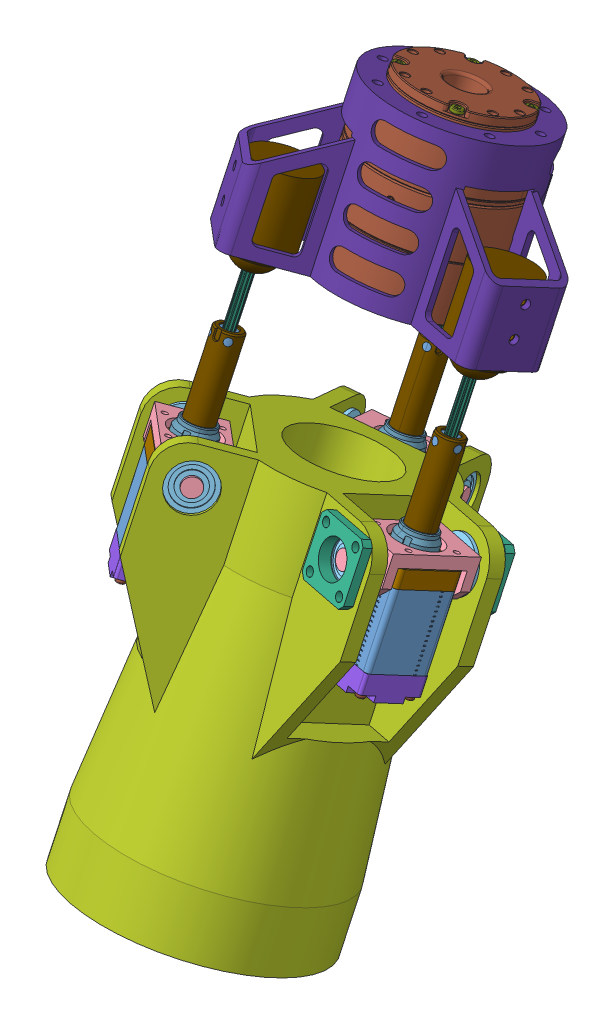
SolidWorks assembly 机械臂总装, configuration 默认. Lengths in mm.
Overall size (121.27 258.43 202.88).
175 component instances, 61 part files, 56 mates.
Components (placement in the parent):
- CRA-RI40-52-PRO-XX 2023.5.4 - Drum-1: CRA-RI40-52-PRO-XX 2023.5.4 - Drum [默认] at (-65.3352 0.778 -52.4868) x (-0.773511 0.267701 0.574471) z (-0.632199 -0.261859 -0.729215) size (67.95 60.31 67.96)
  - CRA-RI40-52-PRO-XX 2023.5.4 - Drum.stp-1: CRA-RI40-52-PRO-XX 2023.5.4 - Drum.stp [默认] at origin size (67.95 60.31 67.96)
    - CRA-RI40-52-PRO-XX_1_ASM.stp-1: CRA-RI40-52-PRO-XX_1_ASM.stp [默认] at origin size (67.95 60.31 67.96)
      - XB11-52__10001_ASM.stp-1: XB11-52__10001_ASM.stp [默认] at (0 16.8 0) x (0.703875 0 -0.710324) z (-0.710324 0 -0.703875) size (66.32 0.8 66.32)
        - XB11-52-06__10001.stp-1: XB11-52-06__10001.stp [默认] at (0 15.8 0) x (0.791272 0 -0.611464) z (-0.611464 0 -0.791272) size (47.28 0.81 47.28)
      - TINYMBS20WITHCONNECTOR2_ASM.stp-1: TINYMBS20WITHCONNECTOR2_ASM.stp [默认] at (2.7275 -27.9719 -6.5848) x (0 -1 0) z (0.92388 0 0.382683) size (0.82 3.25 5.53)
        - FH34SRJ8S05SH_STEP_STEP_ASM.stp-1: FH34SRJ8S05SH_STEP_STEP_ASM.stp [默认] at (-6.4719 -22.2833 0) x (0 0 -1) z (1 0 0) size (5.53 3.25 0.82)
          - NONE-51348.stp-1: NONE-51348.stp [默认] at origin size (0.15 0.3 0.08)
          - NONE-53783.stp-1: NONE-53783.stp [默认] at origin size (0.15 0.3 0.08)
          - NONE-55744.stp-1: NONE-55744.stp [默认] at origin size (0.15 0.08 0.08)
          - NONE-57763.stp-1: NONE-57763.stp [默认] at origin size (0.15 0.08 0.08)
          - NONE-60582.stp-1: NONE-60582.stp [默认] at origin size (0.15 0.3 0.08)
          - NONE-60979.stp-1: NONE-60979.stp [默认] at origin size (0.15 0.3 0.08)
          - NONE-62950.stp-1: NONE-62950.stp [默认] at origin size (0.15 0.3 0.08)
          - NONE-64179.stp-1: NONE-64179.stp [默认] at origin size (0.15 0.3 0.08)
          - NONE-65774.stp-1: NONE-65774.stp [默认] at origin size (0.15 0.08 0.08)
          - NONE-66548.stp-1: NONE-66548.stp [默认] at origin size (0.15 0.35 0.23)
          - NONE-67775.stp-1: NONE-67775.stp [默认] at origin size (0.15 0.35 0.23)
          - NONE-133224.stp-1: NONE-133224.stp [默认] at origin size (0.15 0.08 0.08)
          - NONE-134873.stp-1: NONE-134873.stp [默认] at origin size (0.15 0.3 0.08)
          - NONE-136443.stp-1: NONE-136443.stp [默认] at origin size (0.15 0.08 0.08)
          - NONE-141250.stp-1: NONE-141250.stp [默认] at origin size (0.15 0.35 0.23)
          - NONE-145287.stp-1: NONE-145287.stp [默认] at origin size (0.15 0.08 0.08)
          - NONE-147294.stp-1: NONE-147294.stp [默认] at origin size (0.15 0.08 0.08)
          - NONE-214429.stp-1: NONE-214429.stp [默认] at origin size (0.15 0.9 0.82)
          - NONE-214822.stp-1: NONE-214822.stp [默认] at origin size (0.15 0.3 0.08)
          - NONE-215190.stp-1: NONE-215190.stp [默认] at origin size (0.15 0.08 0.08)
          - NONE-216041.stp-1: NONE-216041.stp [默认] at origin size (0.15 0.35 0.23)
          - NONE-217624.stp-1: NONE-217624.stp [默认] at origin size (0.15 0.35 0.23)
          - NONE-222885.stp-1: NONE-222885.stp [默认] at origin size (0.15 0.35 0.23)
          - NONE-224875.stp-1: NONE-224875.stp [默认] at origin size (0.15 0.35 0.23)
          - NONE-228113.stp-1: NONE-228113.stp [默认] at origin size (0.15 0.9 0.82)
          - NONE-228916.stp-1: NONE-228916.stp [默认] at origin size (0.15 0.35 0.23)
      - CROSS_RECESSED_COUNTERSUNK_HE_1.stp-1: CROSS_RECESSED_COUNTERSUNK_HE_1.stp [默认] at (-21.8123 -33.1 2.8703) x (0 1 0) z (0.6 0 0.8) size (4 3.5 3.5)
      - RI40-52-D12-02__1000.stp-1: RI40-52-D12-02__1000.stp [默认] at (0 -15 0) x (0.382683 0 -0.92388) z (0.92388 0 0.382683) size (52.01 56.6 52)
      - CROSS_RECESSED_CHEESE_HEAD_SC_1.stp-1: CROSS_RECESSED_CHEESE_HEAD_SC_1.stp [默认] at (3.9505 15.5 -22.4044) x (0 -1 0) z (1 0 0) size (5.7 2.98 2.98)
      - MC50-D25X12_5_000.stp-1: MC50-D25X12_5_000.stp [默认] at (0.0001 -26.6014 0.0001) x (0.382686 0 -0.923879) z (0 -1 0) size (48.11 50.01 13.43)
      - CROSS_RECESSED_CHEESE_HEAD_SC_1.stp-2: CROSS_RECESSED_CHEESE_HEAD_SC_1.stp [默认] at (-3.9505 15.5 22.4044) x (0 -1 0) z (-1 0 0) size (5.7 2.98 2.98)
      - CROSS_RECESSED_COUNTERSUNK_HE_1.stp-2: CROSS_RECESSED_COUNTERSUNK_HE_1.stp [默认] at (-3.0048 -33.1 22.5417) x (0 1 0) z (0.395734 0 0.918365) size (4 3.5 3.5)
      - CROSS_RECESSED_CHEESE_HEAD_SC_1.stp-3: CROSS_RECESSED_CHEESE_HEAD_SC_1.stp [默认] at (-18.6357 15.5 13.0489) x (0 -1 0) z (-0.707107 0 -0.707107) size (5.7 2.98 2.98)
      - CROSS_RECESSED_COUNTERSUNK_HE_1.stp-3: CROSS_RECESSED_COUNTERSUNK_HE_1.stp [默认] at (18.8645 -33.1 -12.4259) x (0 1 0) z (0.188455 0 0.982082) size (4 3.5 3.5)
      - _M2X3_M2X3_100.stp-1: _M2X3_M2X3_100.stp [默认] at (-21.8118 -29.6014 2.8705) x (0.8 0 -0.6) z (0.6 0 0.8) size (3.23 5.8 2.8)
      - _M2X3_M2X3_100.stp-2: _M2X3_M2X3_100.stp [默认] at (-13.393 -29.6014 -17.4539) x (0.918365 0 -0.395734) z (0.395734 0 0.918365) size (3.23 5.8 2.8)
      - CROSS_RECESSED_CHEESE_HEAD_SC_1.stp-4: CROSS_RECESSED_CHEESE_HEAD_SC_1.stp [默认] at (-22.4044 15.5 -3.9505) x (0 -1 0) z (0 0 -1) size (5.7 2.98 2.98)
      - CROSS_RECESSED_CHEESE_HEAD_SC_1.stp-5: CROSS_RECESSED_CHEESE_HEAD_SC_1.stp [默认] at (13.0489 15.5 18.6357) x (0 -1 0) z (-0.707107 0 0.707107) size (5.7 2.98 2.98)
      - HEXAGON_SOCKET_HEAD_CAP_SCREW_1.stp-1: HEXAGON_SOCKET_HEAD_CAP_SCREW_1.stp [默认] at (19.8197 15.9 12.6265) x (0 -1 0) z (-0.954517 0 0.298155) size (22.5 4.5 4.5)
      - M2-3_10001.stp-1: M2-3_10001.stp [默认] at (0.7742 21 -17.7331) x (0.020141 0 0.999797) z (-0.999797 0 0.020141) size (4 5.4 4)
      - HEXAGON_SOCKET_HEAD_CAP_SCREW_1.stp-2: HEXAGON_SOCKET_HEAD_CAP_SCREW_1.stp [默认] at (-19.8197 15.9 -12.6265) x (0 -1 0) z (0.954517 0 -0.298155) size (22.5 4.5 4.5)
      - CROSS_RECESSED_CHEESE_HEAD_SC_1.stp-6: CROSS_RECESSED_CHEESE_HEAD_SC_1.stp [默认] at (18.6357 15.5 -13.0489) x (0 -1 0) z (0.707107 0 0.707107) size (5.7 2.98 2.98)
      - M2-3_10001.stp-2: M2-3_10001.stp [默认] at (-17.7331 21 -0.7742) x (0.999797 0 -0.020141) z (0.020141 0 0.999797) size (4 5.4 4)
      - _M2X3_M2X3_100.stp-3: _M2X3_M2X3_100.stp [默认] at (-3.0038 -29.6014 22.5414) x (0.982082 0 -0.188455) z (0.188455 0 0.982082) size (3.23 5.8 2.8)
      - M2-3_10001.stp-3: M2-3_10001.stp [默认] at (-0.7742 21 17.7331) x (-0.020141 0 -0.999797) z (0.999797 0 -0.020141) size (4 5.4 4)
      - _M2X3_M2X3_100.stp-4: _M2X3_M2X3_100.stp [默认] at (18.8646 -29.6014 -12.4267) size (3.23 5.8 2.8)
      - CROSS_RECESSED_COUNTERSUNK_HE_1.stp-4: CROSS_RECESSED_COUNTERSUNK_HE_1.stp [默认] at (-13.393 -33.1 -17.4539) x (0 1 0) z (0 0 1) size (4 3.5 3.5)
      - M2-3_10001.stp-4: M2-3_10001.stp [默认] at (17.7331 21 0.7742) x (-0.999797 0 0.020141) z (-0.020141 0 -0.999797) size (4 5.4 4)
      - CROSS_RECESSED_CHEESE_HEAD_SC_1.stp-7: CROSS_RECESSED_CHEESE_HEAD_SC_1.stp [默认] at (22.4044 15.5 3.9505) x (0 -1 0) z (0 0 1) size (5.7 2.98 2.98)
      - CROSS_RECESSED_CHEESE_HEAD_SC_1.stp-8: CROSS_RECESSED_CHEESE_HEAD_SC_1.stp [默认] at (-13.0489 15.5 -18.6357) x (0 -1 0) z (0.707107 0 -0.707107) size (5.7 2.98 2.98)
- 手腕电机座-1: 手腕电机座 [默认] at (-66.8577 -30.748 -39.8459) x (-0.288066 -0.344371 -0.893547) z (0.956563 -0.147114 -0.251684) size (84.79 53 96.67)
- 球铰2-1: 球铰2 [默认] at (-91.8577 2.9201 -23.4423) x (-0.727754 -0.224677 -0.647992) z (-0.684375 0.29959 0.664738) size (21 30.5 20.4)
- 球铰2-2: 球铰2 [默认] at (-28.733 -6.7882 -40.0512) x (-0.228809 0.371791 0.899677) z (0.972441 0.044781 0.228809) size (21 30.5 20.4)
- 球铰2-3: 球铰2 [默认] at (-76.7583 -21.6149 -82.813) x (0.956563 -0.147114 -0.251684) z (-0.288066 -0.344371 -0.893547) size (21 30.5 20.4)
- 20NC38..31-1: 20NC38..31 [默认] at (-34.2487 -117.8316 4.4347) x (0.046372 0.927308 -0.371416) z (0.972366 0.043263 0.229417) size (109.8 25.88 45.74)
  - 20NC38..31.STEP-1: 20NC38..31.STEP [默认] at origin size (109.8 25.88 45.74)
    - 02-20-38.15________.STEP-1: 02-20-38.15________.STEP [默认] at origin size (39.65 25.88 45.74)
      - 02-20-38.STEP-1: 02-20-38.STEP [默认] at (20.075 0 0) x (0 0 1) z (-1 0 0) size (26.04 25.88 31.46)
        - 02-20-24.15_10-20-001-2.STEP-1: 02-20-24.15_10-20-001-2.STEP [默认] at origin size (20 20 24.15)
        - 13-20-8.5____.STEP-1: 13-20-8.5____.STEP [默认] at (0 0 16.075) x (0 1 0) z (0 0 -1) size (18.2 22.2 10.51)
        - 13-20-12.5______.STEP-1: 13-20-12.5______.STEP [默认] at (0 0 -14.575) x (0.707107 0.707107 0) z (0 0 1) size (18.3 18.3 15.8)
      - 03-20-008______38_______default.STEP-1: 03-20-008______38_______default.STEP [默认] at (3.8 0 0) x (1 0 0) z (0 0.78069 0.624918) size (32.3 16.26 16.27)
        - 06-20-008______38_________01-20-007-1.STEP-1: 06-20-008______38_________01-20-007-1.STEP [默认] at origin size (32.3 7 7)
        - 03-20-4.2-6YK_10-20-006-2.STEP-1: 03-20-4.2-6YK_10-20-006-2.STEP [默认] at (24.2 0 0) x (0 0.91534 0.402682) z (-1 0 0) size (12.06 12.08 4.24)
        - 10-20-001__________.STEP-1: 10-20-001__________.STEP [默认] at (16.9 0 0) x (0 0 1) z (-1 0 0) size (11 11 1)
        - 08-20-001______1_______07-20-001-1.STEP-1: 08-20-001______1_______07-20-001-1.STEP [默认] at (22.1 0 0) x (0 0 1) z (-1 0 0) size (11 11 1)
        - 08-20-001______1_______07-20-001-1.STEP-2: 08-20-001______1_______07-20-001-1.STEP [默认] at (11.4 0 0) x (0 0 1) z (-1 0 0) size (11 11 1)
        - 03-20-4.2-6YK_10-20-006-2.STEP-2: 03-20-4.2-6YK_10-20-006-2.STEP [默认] at (19 0 0) x (0 0.888249 0.459362) z (-1 0 0) size (12.06 12.08 4.24)
        - 03-20-4.2-6YK_10-20-006-2.STEP-3: 03-20-4.2-6YK_10-20-006-2.STEP [默认] at (13.5 0 0) x (0 0.91534 0.402682) z (-1 0 0) size (12.06 12.08 4.24)
        - 03-20-4.2-6YK_10-20-006-2.STEP-4: 03-20-4.2-6YK_10-20-006-2.STEP [默认] at (8.3 0 0) x (0 0.888249 0.459362) z (-1 0 0) size (12.06 12.08 4.24)
      - 01-20-003__20__________________.STEP-1: 01-20-003__20__________________.STEP [默认] at origin size (8.8 20 20)
      - 01-20-001__20__________________.STEP-1: 01-20-001__20__________________.STEP [默认] at (31.35 0 0) x (0 0 1) z (1 0 0) size (20 20 8.3)
      - 09-20-001____9X__5X4)_09-20-001.STEP-1: 09-20-001____9X__5X4)_09-20-001.STEP [默认] at (33.1 0 0) x (1 0 0) z (0 0.994502 0.104719) size (3 9 9)
      - 09-20-001____9X__5X4)_09-20-001.STEP-2: 09-20-001____9X__5X4)_09-20-001.STEP [默认] at (3.8 0 0) x (1 0 0) z (0 -0.49427 -0.869308) size (3 9 9)
      - 11-20-002__M2-37__20-42__.STEP-1: 11-20-002__M2-37__20-42__.STEP [默认] at (0.39 -7.7 7.7) x (0 0 -1) z (1 0 0) size (3 3 33)
      - 11-20-002__M2-37__20-42__.STEP-2: 11-20-002__M2-37__20-42__.STEP [默认] at (0.39 -7.7 -7.7) x (0 1 0) z (1 0 0) size (3 3 33)
      - 11-20-002__M2-37__20-42__.STEP-3: 11-20-002__M2-37__20-42__.STEP [默认] at (0.39 7.7 -7.7) x (0 0 1) z (1 0 0) size (3 3 33)
      - 11-20-002__M2-37__20-42__.STEP-4: 11-20-002__M2-37__20-42__.STEP [默认] at (0.39 7.7 7.7) x (0 -1 0) z (1 0 0) size (3 3 33)
      - 06-20-099__20___________20____________YK.STEP-1: 06-20-099__20___________20____________YK.STEP [默认] at (31.1 0 0) x (0 -0.624918 0.78069) z (-1 0 0) size (6.01 6.01 10)
      - 14-20-001__20-28____________________.STEP-1: 14-20-001__20-28____________________.STEP [默认] at (6.15 0 -8.6) x (0 -1 0) z (0 0 1) size (10.5 3.4 24.5)
    - 07-20-007__________________.STEP-1: 07-20-007__________________.STEP [默认] at (39.65 0 0) x (-1 0 0) z (0 -0.999857 -0.016895) size (6 12.92 13)
    - 07-20-013-2______________.STEP-1: 07-20-013-2______________.STEP [默认] at (68.4 0 0) x (0 -0.714016 0.700129) z (1 0 0) size (3.42 3.5 41.4)
    - 07-20-013-3______________.STEP-1: 07-20-013-3______________.STEP [默认] at (20.15 0 0) x (0 0.924225 0.381849) z (1 0 0) size (8 8 56.63)
    - 07-20-006__20______.STEP-1: 07-20-006__20______.STEP [默认] at (67.9 0 0) x (0 0.924225 0.381849) z (1 0 0) size (3.9 4.45 0.4)
    - 07-20-013-1__20_____________08-20-002-1.STEP-1: 07-20-013-1__20_____________08-20-002-1.STEP [默认] at (36.1 0 0) x (0 0.004204 -0.999991) z (1 0 0) size (9.01 9.01 35.91)
    - 07-20-002__20________________.STEP-1: 07-20-002__20________________.STEP [默认] at (69.65 0 0) x (0 0.004204 -0.999991) z (1 0 0) size (9.01 9.01 3.1)
- 螺纹转换套-1: 螺纹转换套 [默认] at (-30.0844 -34.5593 -28.9185) x (-0.195243 -0.356231 -0.913772) z (0.046372 0.927308 -0.371416) size (5 5 5)
- 球-1: 球 [默认] at (-29.7853 -28.5782 -31.3141) x (-0.55453 -0.285367 -0.781705) z (0.830871 -0.242211 -0.500987) size (14 13.45 14)
- 球-2: 球 [默认] at (-92.91 -18.87 -14.7052) x (0.833324 -0.238487 -0.498693) z (0.551058 0.287142 0.783508) size (14 13.45 14)
- 螺纹转换套-2: 螺纹转换套 [默认] at (-78.0965 -49.3819 -71.6684) x (0.952783 0.073148 0.29471) z (0.044309 0.926671 -0.373253) size (5 5 5)
- 螺纹转换套-3: 螺纹转换套 [默认] at (-93.1916 -24.8538 -12.3142) x (-0.196131 -0.355877 -0.91372) z (0.043661 0.927725 -0.370703) size (5 5 5)
- 球-3: 球 [默认] at (-77.8107 -43.4049 -74.0759) x (0.898492 0.126374 0.420407) z (-0.436749 0.353993 0.827006) size (14 13.45 14)
- 20NC38..31-2: 20NC38..31 [默认] at (-82.0754 -132.597 -38.1503) x (0.044309 0.926671 -0.373253) z (-0.288139 -0.345888 -0.892937) size (109.8 25.88 45.74)
  - 20NC38..31.STEP-1: 20NC38..31.STEP [默认] at origin size (109.8 25.88 45.74)
    - 02-20-38.15________.STEP-1: 02-20-38.15________.STEP [默认] at origin size (39.65 25.88 45.74)
      - 02-20-38.STEP-1: 02-20-38.STEP [默认] at (20.075 0 0) x (0 0 1) z (-1 0 0) size (26.04 25.88 31.46)
        - 02-20-24.15_10-20-001-2.STEP-1: 02-20-24.15_10-20-001-2.STEP [默认] at origin size (20 20 24.15)
        - 13-20-8.5____.STEP-1: 13-20-8.5____.STEP [默认] at (0 0 16.075) x (0 1 0) z (0 0 -1) size (18.2 22.2 10.51)
        - 13-20-12.5______.STEP-1: 13-20-12.5______.STEP [默认] at (0 0 -14.575) x (0.707107 0.707107 0) z (0 0 1) size (18.3 18.3 15.8)
      - 03-20-008______38_______default.STEP-1: 03-20-008______38_______default.STEP [默认] at (3.8 0 0) x (1 0 0) z (0 0.78069 0.624918) size (32.3 16.26 16.27)
        - 06-20-008______38_________01-20-007-1.STEP-1: 06-20-008______38_________01-20-007-1.STEP [默认] at origin size (32.3 7 7)
        - 03-20-4.2-6YK_10-20-006-2.STEP-1: 03-20-4.2-6YK_10-20-006-2.STEP [默认] at (24.2 0 0) x (0 0.91534 0.402682) z (-1 0 0) size (12.06 12.08 4.24)
        - 10-20-001__________.STEP-1: 10-20-001__________.STEP [默认] at (16.9 0 0) x (0 0 1) z (-1 0 0) size (11 11 1)
        - 08-20-001______1_______07-20-001-1.STEP-1: 08-20-001______1_______07-20-001-1.STEP [默认] at (22.1 0 0) x (0 0 1) z (-1 0 0) size (11 11 1)
        - 08-20-001______1_______07-20-001-1.STEP-2: 08-20-001______1_______07-20-001-1.STEP [默认] at (11.4 0 0) x (0 0 1) z (-1 0 0) size (11 11 1)
        - 03-20-4.2-6YK_10-20-006-2.STEP-2: 03-20-4.2-6YK_10-20-006-2.STEP [默认] at (19 0 0) x (0 0.888249 0.459362) z (-1 0 0) size (12.06 12.08 4.24)
        - 03-20-4.2-6YK_10-20-006-2.STEP-3: 03-20-4.2-6YK_10-20-006-2.STEP [默认] at (13.5 0 0) x (0 0.91534 0.402682) z (-1 0 0) size (12.06 12.08 4.24)
        - 03-20-4.2-6YK_10-20-006-2.STEP-4: 03-20-4.2-6YK_10-20-006-2.STEP [默认] at (8.3 0 0) x (0 0.888249 0.459362) z (-1 0 0) size (12.06 12.08 4.24)
      - 01-20-003__20__________________.STEP-1: 01-20-003__20__________________.STEP [默认] at origin size (8.8 20 20)
      - 01-20-001__20__________________.STEP-1: 01-20-001__20__________________.STEP [默认] at (31.35 0 0) x (0 0 1) z (1 0 0) size (20 20 8.3)
      - 09-20-001____9X__5X4)_09-20-001.STEP-1: 09-20-001____9X__5X4)_09-20-001.STEP [默认] at (33.1 0 0) x (1 0 0) z (0 0.994502 0.104719) size (3 9 9)
      - 09-20-001____9X__5X4)_09-20-001.STEP-2: 09-20-001____9X__5X4)_09-20-001.STEP [默认] at (3.8 0 0) x (1 0 0) z (0 -0.49427 -0.869308) size (3 9 9)
      - 11-20-002__M2-37__20-42__.STEP-1: 11-20-002__M2-37__20-42__.STEP [默认] at (0.39 -7.7 7.7) x (0 0 -1) z (1 0 0) size (3 3 33)
      - 11-20-002__M2-37__20-42__.STEP-2: 11-20-002__M2-37__20-42__.STEP [默认] at (0.39 -7.7 -7.7) x (0 1 0) z (1 0 0) size (3 3 33)
      - 11-20-002__M2-37__20-42__.STEP-3: 11-20-002__M2-37__20-42__.STEP [默认] at (0.39 7.7 -7.7) x (0 0 1) z (1 0 0) size (3 3 33)
      - 11-20-002__M2-37__20-42__.STEP-4: 11-20-002__M2-37__20-42__.STEP [默认] at (0.39 7.7 7.7) x (0 -1 0) z (1 0 0) size (3 3 33)
      - 06-20-099__20___________20____________YK.STEP-1: 06-20-099__20___________20____________YK.STEP [默认] at (31.1 0 0) x (0 -0.624918 0.78069) z (-1 0 0) size (6.01 6.01 10)
      - 14-20-001__20-28____________________.STEP-1: 14-20-001__20-28____________________.STEP [默认] at (6.15 0 -8.6) x (0 -1 0) z (0 0 1) size (10.5 3.4 24.5)
    - 07-20-007__________________.STEP-1: 07-20-007__________________.STEP [默认] at (39.65 0 0) x (-1 0 0) z (0 -0.999857 -0.016895) size (6 12.92 13)
    - 07-20-013-2______________.STEP-1: 07-20-013-2______________.STEP [默认] at (68.4 0 0) x (0 -0.714016 0.700129) z (1 0 0) size (3.42 3.5 41.4)
    - 07-20-013-3______________.STEP-1: 07-20-013-3______________.STEP [默认] at (20.15 0 0) x (0 0.924225 0.381849) z (1 0 0) size (8 8 56.63)
    - 07-20-006__20______.STEP-1: 07-20-006__20______.STEP [默认] at (67.9 0 0) x (0 0.924225 0.381849) z (1 0 0) size (3.9 4.45 0.4)
    - 07-20-013-1__20_____________08-20-002-1.STEP-1: 07-20-013-1__20_____________08-20-002-1.STEP [默认] at (36.1 0 0) x (0 0.004204 -0.999991) z (1 0 0) size (9.01 9.01 35.91)
    - 07-20-002__20________________.STEP-1: 07-20-002__20________________.STEP [默认] at (69.65 0 0) x (0 0.004204 -0.999991) z (1 0 0) size (9.01 9.01 3.1)
- 20NC38..31-3: 20NC38..31 [默认] at (-97.1124 -108.1635 20.9749) x (0.043661 0.927725 -0.370703) z (-0.684447 0.298072 0.665346) size (109.8 25.88 45.74)
  - 20NC38..31.STEP-1: 20NC38..31.STEP [默认] at origin size (109.8 25.88 45.74)
    - 02-20-38.15________.STEP-1: 02-20-38.15________.STEP [默认] at origin size (39.65 25.88 45.74)
      - 02-20-38.STEP-1: 02-20-38.STEP [默认] at (20.075 0 0) x (0 0 1) z (-1 0 0) size (26.04 25.88 31.46)
        - 02-20-24.15_10-20-001-2.STEP-1: 02-20-24.15_10-20-001-2.STEP [默认] at origin size (20 20 24.15)
        - 13-20-8.5____.STEP-1: 13-20-8.5____.STEP [默认] at (0 0 16.075) x (0 1 0) z (0 0 -1) size (18.2 22.2 10.51)
        - 13-20-12.5______.STEP-1: 13-20-12.5______.STEP [默认] at (0 0 -14.575) x (0.707107 0.707107 0) z (0 0 1) size (18.3 18.3 15.8)
      - 03-20-008______38_______default.STEP-1: 03-20-008______38_______default.STEP [默认] at (3.8 0 0) x (1 0 0) z (0 0.78069 0.624918) size (32.3 16.26 16.27)
        - 06-20-008______38_________01-20-007-1.STEP-1: 06-20-008______38_________01-20-007-1.STEP [默认] at origin size (32.3 7 7)
        - 03-20-4.2-6YK_10-20-006-2.STEP-1: 03-20-4.2-6YK_10-20-006-2.STEP [默认] at (24.2 0 0) x (0 0.91534 0.402682) z (-1 0 0) size (12.06 12.08 4.24)
        - 10-20-001__________.STEP-1: 10-20-001__________.STEP [默认] at (16.9 0 0) x (0 0 1) z (-1 0 0) size (11 11 1)
        - 08-20-001______1_______07-20-001-1.STEP-1: 08-20-001______1_______07-20-001-1.STEP [默认] at (22.1 0 0) x (0 0 1) z (-1 0 0) size (11 11 1)
        - 08-20-001______1_______07-20-001-1.STEP-2: 08-20-001______1_______07-20-001-1.STEP [默认] at (11.4 0 0) x (0 0 1) z (-1 0 0) size (11 11 1)
        - 03-20-4.2-6YK_10-20-006-2.STEP-2: 03-20-4.2-6YK_10-20-006-2.STEP [默认] at (19 0 0) x (0 0.888249 0.459362) z (-1 0 0) size (12.06 12.08 4.24)
        - 03-20-4.2-6YK_10-20-006-2.STEP-3: 03-20-4.2-6YK_10-20-006-2.STEP [默认] at (13.5 0 0) x (0 0.91534 0.402682) z (-1 0 0) size (12.06 12.08 4.24)
        - 03-20-4.2-6YK_10-20-006-2.STEP-4: 03-20-4.2-6YK_10-20-006-2.STEP [默认] at (8.3 0 0) x (0 0.888249 0.459362) z (-1 0 0) size (12.06 12.08 4.24)
      - 01-20-003__20__________________.STEP-1: 01-20-003__20__________________.STEP [默认] at origin size (8.8 20 20)
      - 01-20-001__20__________________.STEP-1: 01-20-001__20__________________.STEP [默认] at (31.35 0 0) x (0 0 1) z (1 0 0) size (20 20 8.3)
      - 09-20-001____9X__5X4)_09-20-001.STEP-1: 09-20-001____9X__5X4)_09-20-001.STEP [默认] at (33.1 0 0) x (1 0 0) z (0 0.994502 0.104719) size (3 9 9)
      - 09-20-001____9X__5X4)_09-20-001.STEP-2: 09-20-001____9X__5X4)_09-20-001.STEP [默认] at (3.8 0 0) x (1 0 0) z (0 -0.49427 -0.869308) size (3 9 9)
      - 11-20-002__M2-37__20-42__.STEP-1: 11-20-002__M2-37__20-42__.STEP [默认] at (0.39 -7.7 7.7) x (0 0 -1) z (1 0 0) size (3 3 33)
      - 11-20-002__M2-37__20-42__.STEP-2: 11-20-002__M2-37__20-42__.STEP [默认] at (0.39 -7.7 -7.7) x (0 1 0) z (1 0 0) size (3 3 33)
      - 11-20-002__M2-37__20-42__.STEP-3: 11-20-002__M2-37__20-42__.STEP [默认] at (0.39 7.7 -7.7) x (0 0 1) z (1 0 0) size (3 3 33)
      - 11-20-002__M2-37__20-42__.STEP-4: 11-20-002__M2-37__20-42__.STEP [默认] at (0.39 7.7 7.7) x (0 -1 0) z (1 0 0) size (3 3 33)
      - 06-20-099__20___________20____________YK.STEP-1: 06-20-099__20___________20____________YK.STEP [默认] at (31.1 0 0) x (0 -0.624918 0.78069) z (-1 0 0) size (6.01 6.01 10)
      - 14-20-001__20-28____________________.STEP-1: 14-20-001__20-28____________________.STEP [默认] at (6.15 0 -8.6) x (0 -1 0) z (0 0 1) size (10.5 3.4 24.5)
    - 07-20-007__________________.STEP-1: 07-20-007__________________.STEP [默认] at (39.65 0 0) x (-1 0 0) z (0 -0.999857 -0.016895) size (6 12.92 13)
    - 07-20-013-2______________.STEP-1: 07-20-013-2______________.STEP [默认] at (68.4 0 0) x (0 -0.714016 0.700129) z (1 0 0) size (3.42 3.5 41.4)
    - 07-20-013-3______________.STEP-1: 07-20-013-3______________.STEP [默认] at (20.15 0 0) x (0 0.924225 0.381849) z (1 0 0) size (8 8 56.63)
    - 07-20-006__20______.STEP-1: 07-20-006__20______.STEP [默认] at (67.9 0 0) x (0 0.924225 0.381849) z (1 0 0) size (3.9 4.45 0.4)
    - 07-20-013-1__20_____________08-20-002-1.STEP-1: 07-20-013-1__20_____________08-20-002-1.STEP [默认] at (36.1 0 0) x (0 0.004204 -0.999991) z (1 0 0) size (9.01 9.01 35.91)
    - 07-20-002__20________________.STEP-1: 07-20-002__20________________.STEP [默认] at (69.65 0 0) x (0 0.004204 -0.999991) z (1 0 0) size (9.01 9.01 3.1)
- 电缸座-1: 电缸座 [默认] at (-95.2721 -69.0599 5.3498) x (0.727754 0.224677 0.647992) z (-0.043661 -0.927725 0.370703) size (42 20 14)
- F696.ZZ-1: F696.ZZ [默认] at (-84.6614 -72.1838 17.6646) x (0.148454 0.870814 -0.468663) z (0.669578 -0.437269 -0.600384) size (17 5 17)
- F696.ZZ-2: F696.ZZ [默认] at (-106.494 -78.9241 -1.7752) x (-0.284553 0.958575 -0.012786) z (-0.624022 -0.175083 0.761539) size (17 5 17)
- 轴承端盖-2: 轴承端盖 [默认] at (-38.1559 -76.2394 13.1516) x (-0.044781 -0.927236 0.371791) z (0.228809 -0.371791 -0.899677) size (20 20 4)
- 轴承端盖-3: 轴承端盖 [默认] at (-27.0815 -94.234 -30.3928) x (-0.044781 -0.927236 0.371791) z (-0.228809 0.371791 0.899677) size (20 20 4)
- 电缸座-4: 电缸座 [默认] at (-32.2941 -78.7455 -11.2205) x (0.228809 -0.371791 -0.899677) z (-0.046372 -0.927308 0.371416) size (42 20 14)
- 电缸座-5: 电缸座 [默认] at (-80.2078 -93.5378 -53.8829) x (-0.956563 0.147114 0.251684) z (-0.044309 -0.926671 0.373253) size (42 20 14)
- 手腕关节-1: 手腕关节 [默认] at (-75.7512 -214.8969 33.9919) x (0.972441 0.044781 0.228809) z (-0.228809 0.371791 0.899677) size (93.36 130 107.8)
- F696.ZZ-7: F696.ZZ [默认] at (-29.1866 -90.8136 -22.1158) x (-0.103795 0.909608 -0.402293) z (-0.967922 -0.18543 -0.169536) size (17 5 17)
- F696.ZZ-9: F696.ZZ [默认] at (-94.8664 -97.8178 -47.4949) x (-0.050847 0.765907 -0.640938) z (0.287058 0.625895 0.725158) size (17 5 17)
- F696.ZZ-10: F696.ZZ [默认] at (-66.1695 -102.2312 -55.0454) x (-0.036507 0.796088 -0.604079) z (-0.289231 -0.587028 -0.756137) size (17 5 17)
- F696.ZZ-11: F696.ZZ [默认] at (-36.0508 -79.6598 4.8745) x (-0.228512 0.877857 -0.42089) z (0.946271 0.30189 0.115903) size (17 5 17)
Mates (geometry in assembly coordinates):
- 重合2: coincident anti-aligned: plane of 手腕电机座-1 through (-91.4115 21.8166 -16.6063) normal (0.684375 -0.29959 -0.664738); plane of 球铰2-1 through (-98.102 -35.0535 2.1363) normal (-0.684375 0.29959 0.664738)
- 同心6: concentric aligned: cylinder of 手腕电机座-1 through (-93.3819 -1.1469 -20.3204) axis (-0.684375 0.29959 0.664738) radius 1.5; cylinder of 球铰2-1 through (-92.0131 -1.7461 -21.6498) axis (-0.684375 0.29959 0.664738) radius 1.25
- 同心7: concentric anti-aligned: cylinder of 20NC38..31-1/20NC38..31.STEP-1/07-20-013-2______________.STEP-1 through (-29.3889 -20.6497 -34.4897) axis (0.046372 0.927308 -0.371416) radius 1.25; cylinder of 螺纹转换套-1 through (-29.8526 -29.9228 -30.7756) axis (-0.046372 -0.927308 0.371416) radius 1.25
- 同心8: concentric aligned: cylinder of 螺纹转换套-1 through (-29.8526 -29.9228 -30.7756) axis (-0.046372 -0.927308 0.371416) radius 2.5; cylinder of 球-1 through (-29.8526 -29.9228 -30.7756) axis (-0.046372 -0.927308 0.371416) radius 2.5
- 重合3: coincident anti-aligned: plane of 螺纹转换套-1 through (-29.8526 -29.9228 -30.7756) normal (0.046372 0.927308 -0.371416); plane of 球-1 through (-29.8526 -29.9228 -30.7756) normal (-0.046372 -0.927308 0.371416)
- 同心10: concentric aligned: cylinder of 手腕电机座-1 through (-93.8297 -10.4192 -16.6024) axis (-0.684375 0.29959 0.664738) radius 1.5; cylinder of 球铰2-1 through (-92.4609 -11.0184 -17.9319) axis (-0.684375 0.29959 0.664738) radius 1.25
- 同心11: concentric anti-aligned: cylinder of 螺纹转换套-2 through (-77.8749 -44.7486 -73.5347) axis (-0.044309 -0.926671 0.373253) radius 2.5; cylinder of 20NC38..31-2/20NC38..31.STEP-1/07-20-013-2______________.STEP-1 through (-77.4318 -35.4819 -77.2672) axis (0.044309 0.926671 -0.373253) radius 1.25
- 同心12: concentric aligned: cylinder of 螺纹转换套-2 through (-77.8749 -44.7486 -73.5347) axis (-0.044309 -0.926671 0.373253) radius 2.5; cylinder of 球-3 through (-77.8749 -44.7486 -73.5347) axis (-0.044309 -0.926671 0.373253) radius 2.5
- 重合4: coincident anti-aligned: plane of 螺纹转换套-2 through (-77.8749 -44.7486 -73.5347) normal (0.044309 0.926671 -0.373253); plane of 球-3 through (-77.8749 -44.7486 -73.5347) normal (-0.044309 -0.926671 0.373253)
- 同心13: concentric anti-aligned: cylinder of 螺纹转换套-3 through (-92.9733 -20.2152 -14.1677) axis (-0.043661 -0.927725 0.370703) radius 2.5; axis of 20NC38..31-3/20NC38..31.STEP-1/07-20-013-2______________.STEP-1 through (-92.5367 -10.9379 -17.8747) axis (0.043661 0.927725 -0.370703)
- 同心14: concentric aligned: cylinder of 球-2 through (-92.9733 -20.2152 -14.1677) axis (-0.043661 -0.927725 0.370703) radius 2.5; cylinder of 螺纹转换套-3 through (-92.9733 -20.2152 -14.1677) axis (-0.043661 -0.927725 0.370703) radius 2.5
- 重合5: coincident anti-aligned: plane of 球-2 through (-92.9733 -20.2152 -14.1677) normal (-0.043661 -0.927725 0.370703); plane of 螺纹转换套-3 through (-92.9733 -20.2152 -14.1677) normal (0.043661 0.927725 -0.370703)
- 重合6: coincident anti-aligned: plane of 20NC38..31-3/20NC38..31.STEP-1/02-20-38.15________.STEP-1/01-20-001__20__________________.STEP-1 through (-95.0786 -68.3274 17.996) normal (0.043661 0.927725 -0.370703); plane of 电缸座-1 through (-95.4467 -72.7708 6.8326) normal (-0.043661 -0.927725 0.370703)
- 同心17: concentric aligned: cylinder of 20NC38..31-3/20NC38..31.STEP-1/02-20-38.15________.STEP-1/01-20-001__20__________________.STEP-1 through (-95.4467 -72.7708 6.8326) axis (0.043661 0.927725 -0.370703) radius 8; cylinder of 电缸座-1 through (-95.4467 -72.7708 6.8326) axis (0.043661 0.927725 -0.370703) radius 8
- 同心18: concentric anti-aligned: cylinder of 20NC38..31-3/20NC38..31.STEP-1/02-20-38.15________.STEP-1/01-20-001__20__________________.STEP-1 through (-84.5073 -71.9443 6.1429) axis (-0.043661 -0.927725 0.370703) radius 0.75; line of 电缸座-1 through (-84.5727 -73.3359 6.699) axis (0.043661 0.927725 -0.370703)
- 同心19: concentric anti-aligned: cylinder of 电缸座-1 through (-80.2948 -70.8357 21.5526) axis (-0.727754 -0.224677 -0.647992) radius 3; cylinder of F696.ZZ-1 through (-79.4147 -70.564 22.3363) axis (0.727754 0.224677 0.647992) radius 3
- 重合7: coincident anti-aligned: plane of 电缸座-1 through (-84.3557 -65.6897 15.0697) normal (0.727754 0.224677 0.647992); plane of F696.ZZ-1 through (-83.9933 -68.2651 15.5556) normal (-0.727754 -0.224677 -0.647992)
- 同心20: concentric anti-aligned: cylinder of F696.ZZ-1 through (-79.4147 -70.564 22.3363) axis (0.727754 0.224677 0.647992) radius 7.5; cylinder of F696.ZZ-2 through (-111.7407 -80.5439 -6.4468) axis (-0.727754 -0.224677 -0.647992) radius 7.5
- 重合8: coincident anti-aligned: plane of 电缸座-1 through (-106.1884 -72.43 -4.3701) normal (-0.727754 -0.224677 -0.647992); plane of F696.ZZ-2 through (-108.9127 -70.7762 -1.8838) normal (0.727754 0.224677 0.647992)
- 同心33: concentric anti-aligned: cylinder of F696.ZZ-6 through (-2.5623 -103.2131 137.2832) axis (-0.228809 0.371791 0.899677) radius 3; cylinder of 电缸座-4 through (-37.4237 -77.4291 10.2726) axis (0.228809 -0.371791 -0.899677) radius 3
- 重合17: coincident anti-aligned: plane of 20NC38..31-1/20NC38..31.STEP-1/02-20-38.15________.STEP-1/01-20-001__20__________________.STEP-1 through (-22.2696 -85.2473 -15.4321) normal (0.046372 0.927308 -0.371416); plane of 电缸座-4 through (-32.4796 -82.4548 -9.7349) normal (-0.046372 -0.927308 0.371416)
- 同心35: concentric anti-aligned: cylinder of 20NC38..31-1/20NC38..31.STEP-1/02-20-38.15________.STEP-1/01-20-001__20__________________.STEP-1 through (-38.1354 -84.2597 -18.986) axis (-0.046372 -0.927308 0.371416) radius 0.75; cylinder of 电缸座-4 through (-38.205 -85.6507 -18.4289) axis (0.046372 0.927308 -0.371416) radius 1
- 同心36: concentric anti-aligned: cylinder of 20NC38..31-1/20NC38..31.STEP-1/02-20-38.15________.STEP-1/01-20-001__20__________________.STEP-1 through (-41.6591 -78.5342 -5.131) axis (-0.046372 -0.927308 0.371416) radius 0.75; cylinder of 电缸座-4 through (-41.7286 -79.9251 -4.5739) axis (0.046372 0.927308 -0.371416) radius 1
- 重合18: coincident anti-aligned: plane of 20NC38..31-2/20NC38..31.STEP-1/02-20-38.15________.STEP-1/01-20-001__20__________________.STEP-1 through (-90.965 -98.934 -57.8405) normal (0.044309 0.926671 -0.373253); plane of 电缸座-5 through (-80.385 -97.2445 -52.3899) normal (-0.044309 -0.926671 0.373253)
- 同心38: concentric aligned: cylinder of 20NC38..31-2/20NC38..31.STEP-1/02-20-38.15________.STEP-1/01-20-001__20__________________.STEP-1 through (-80.385 -97.2445 -52.3899) axis (0.044309 0.926671 -0.373253) radius 8; cylinder of 电缸座-5 through (-80.385 -97.2445 -52.3899) axis (0.044309 0.926671 -0.373253) radius 8
- 距离1: distance = 15 mm anti-aligned: plane of 螺纹转换套-2 through (-78.0965 -49.3819 -71.6684) normal (-0.044309 -0.926671 0.373253); plane of 20NC38..31-2/20NC38..31.STEP-1/07-20-013-2______________.STEP-1 through (-77.4318 -35.4819 -77.2672) normal (0.044309 0.926671 -0.373253)
- 距离2: distance = 15 mm anti-aligned: plane of 螺纹转换套-3 through (-93.1916 -24.8538 -12.3142) normal (-0.043661 -0.927725 0.370703); plane of 20NC38..31-3/20NC38..31.STEP-1/07-20-013-2______________.STEP-1 through (-92.5367 -10.9379 -17.8747) normal (0.043661 0.927725 -0.370703)
- 距离3: distance = 15 mm anti-aligned: plane of 螺纹转换套-1 through (-30.0844 -34.5593 -28.9185) normal (-0.046372 -0.927308 0.371416); plane of 20NC38..31-1/20NC38..31.STEP-1/07-20-013-2______________.STEP-1 through (-29.3889 -20.6497 -34.4897) normal (0.046372 0.927308 -0.371416)
- 重合23: coincident anti-aligned: plane of F696.ZZ-6 through (0.831 -101.9217 129.5992) normal (0.228809 -0.371791 -0.899677); plane of 电缸座-4 through (-35.7262 -73.1687 2.2746) normal (-0.228809 0.371791 0.899677)
- 同心48: concentric: sphere of 球铰2-3; sphere of 球-3
- 同心50: concentric anti-aligned: cylinder of 轴承端盖-5 through (7.4846 -119.5382 97.7789) axis (0.228809 -0.371791 -0.899677) radius 6; cylinder of 电缸座-4 through (-27.8137 -93.0443 -27.5138) axis (-0.228809 0.371791 0.899677) radius 3
- 重合24: coincident anti-aligned: plane of 手腕关节-1 through (-68.2381 -142.1049 -12.1852) normal (-0.228809 0.371791 0.899677); plane of F696.ZZ-7 through (-29.6904 -84.4377 -26.2126) normal (0.228809 -0.371791 -0.899677)
- 同心52: concentric anti-aligned: cylinder of 手腕关节-1 through (-27.173 -94.0853 -30.0329) axis (-0.228809 0.371791 0.899677) radius 7.5; cylinder of F696.ZZ-7 through (-27.537 -93.494 -28.6019) axis (0.228809 -0.371791 -0.899677) radius 7.5
- 同心53: concentric anti-aligned: cylinder of 电缸座-4 through (-27.8137 -93.0443 -27.5138) axis (-0.228809 0.371791 0.899677) radius 3; cylinder of F696.ZZ-7 through (-27.537 -93.494 -28.6019) axis (0.228809 -0.371791 -0.899677) radius 3
- 重合25: coincident anti-aligned: plane of 电缸座-4 through (-28.862 -84.3224 -24.7157) normal (0.228809 -0.371791 -0.899677); plane of F696.ZZ-7 through (-30.0688 -83.0819 -25.5352) normal (-0.228809 0.371791 0.899677)
- 同心54: concentric aligned: cylinder of 手腕关节-1 through (-27.173 -94.0853 -30.0329) axis (-0.228809 0.371791 0.899677) radius 7.5; cylinder of F696.ZZ-11 through (-37.7004 -76.9794 11.3607) axis (-0.228809 0.371791 0.899677) radius 7.5
- 重合26: coincident anti-aligned: plane of 手腕关节-1 through (-75.6515 -130.0588 16.9644) normal (0.228809 -0.371791 -0.899677); plane of F696.ZZ-11 through (-38.0392 -72.6298 2.7975) normal (-0.228809 0.371791 0.899677)
- 重合27: coincident anti-aligned: plane of 轴承端盖-2 through (-37.4694 -77.3547 10.4525) normal (0.228809 -0.371791 -0.899677); plane of 手腕关节-1 through (-80.6019 -207.0149 53.065) normal (-0.228809 0.371791 0.899677)
- 平行1: parallel aligned: plane of 轴承端盖-2 through (-38.3251 -52.467 45.522) normal (0.044781 0.927236 -0.371791); plane of 手腕关节-1 through (-69.0341 -75.8115 -21.7768) normal (0.044781 0.927236 -0.371791)
- 同心55: concentric aligned: cylinder of 轴承端盖-2 through (-37.4694 -77.3547 10.4525) axis (-0.228809 0.371791 0.899677) radius 6; cylinder of 手腕关节-1 through (-27.173 -94.0853 -30.0329) axis (-0.228809 0.371791 0.899677) radius 7.5
- 同心56: concentric aligned: circle of 轴承端盖-3; cylinder of 手腕关节-1 through (-27.173 -94.0853 -30.0329) axis (-0.228809 0.371791 0.899677) radius 7.5
- 平行2: parallel aligned: plane of 轴承端盖-3 through (-26.0167 -99.4617 -70.199) normal (0.044781 0.927236 -0.371791); plane of 手腕关节-1 through (-69.0341 -75.8115 -21.7768) normal (0.044781 0.927236 -0.371791)
- 重合30: coincident anti-aligned: plane of 轴承端盖-3 through (-27.7679 -93.1187 -27.6937) normal (-0.228809 0.371791 0.899677); plane of 手腕关节-1 through (-70.9005 -222.7789 14.9187) normal (0.228809 -0.371791 -0.899677)
- 同心57: concentric anti-aligned: cylinder of F696.ZZ-1 through (-79.4147 -70.564 22.3363) axis (0.727754 0.224677 0.647992) radius 7.5; cylinder of 手腕关节-1 through (-78.2571 -70.2066 23.3669) axis (-0.727754 -0.224677 -0.647992) radius 7.5
- 重合32: coincident anti-aligned: plane of F696.ZZ-1 through (-82.6747 -65.3831 14.9272) normal (0.727754 0.224677 0.647992); plane of 手腕关节-1 through (-60.1552 -132.4421 12.8871) normal (-0.727754 -0.224677 -0.647992)
- 同心58: concentric aligned: cylinder of 手腕关节-1 through (-103.2842 -96.5232 -45.28) axis (0.956563 -0.147114 -0.251684) radius 7.5; cylinder of F696.ZZ-10 through (-59.2732 -103.2918 -56.8599) axis (0.956563 -0.147114 -0.251684) radius 7.5
- 重合33: coincident anti-aligned: plane of 手腕关节-1 through (-56.4485 -138.4651 -1.6877) normal (-0.956563 0.147114 0.251684); plane of F696.ZZ-10 through (-65.2954 -96.4371 -59.878) normal (0.956563 -0.147114 -0.251684)
- 同心59: concentric anti-aligned: cylinder of 手腕关节-1 through (-103.2842 -96.5232 -45.28) axis (0.956563 -0.147114 -0.251684) radius 7.5; cylinder of F696.ZZ-9 through (-101.7627 -96.7571 -45.6804) axis (-0.956563 0.147114 0.251684) radius 7.5
- 重合34: coincident anti-aligned: plane of 手腕关节-1 through (-87.4411 -133.6986 6.4669) normal (0.956563 -0.147114 -0.251684); plane of F696.ZZ-9 through (-96.3956 -91.8969 -51.9999) normal (-0.956563 0.147114 0.251684)
- 重合35: coincident anti-aligned: plane of 电缸座-5 through (-65.8594 -95.7445 -57.6582) normal (0.956563 -0.147114 -0.251684); plane of F696.ZZ-10 through (-66.3338 -98.6488 -57.7637) normal (-0.956563 0.147114 0.251684)
- 同心60: concentric anti-aligned: cylinder of 电缸座-5 through (-60.4301 -103.1139 -56.5555) axis (-0.956563 0.147114 0.251684) radius 3; cylinder of F696.ZZ-10 through (-59.2732 -103.2918 -56.8599) axis (0.956563 -0.147114 -0.251684) radius 3
- 同心61: concentric: sphere of 球铰2-1; sphere of 球-2
- 同心63: concentric: sphere of 球铰2-2; sphere of 球-1
- 同心64: concentric anti-aligned: cylinder of 20NC38..31-2/20NC38..31.STEP-1/02-20-38.15________.STEP-1/01-20-001__20__________________.STEP-1 through (-89.9028 -97.385 -57.8874) axis (-0.044309 -0.926671 0.373253) radius 0.75; line of 电缸座-5 through (-89.9692 -98.775 -57.3275) axis (0.044309 0.926671 -0.373253)
- 重合36: coincident anti-aligned: plane of CRA-RI40-52-PRO-XX 2023.5.4 - Drum-1/CRA-RI40-52-PRO-XX 2023.5.4 - Drum.stp-1/CRA-RI40-52-PRO-XX_1_ASM.stp-1/RI40-52-D12-02__1000.stp-1 through (-64.6187 15.6138 -58.4354) normal (0.044781 0.927236 -0.371791); plane of 手腕电机座-1 through (-64.6187 15.6138 -58.4354) normal (-0.044781 -0.927236 0.371791)
- 同心65: concentric aligned: cylinder of CRA-RI40-52-PRO-XX 2023.5.4 - Drum-1/CRA-RI40-52-PRO-XX 2023.5.4 - Drum.stp-1/CRA-RI40-52-PRO-XX_1_ASM.stp-1/RI40-52-D12-02__1000.stp-1 through (-64.9187 9.4013 -55.9444) axis (0.044781 0.927236 -0.371791) radius 20; cylinder of 手腕电机座-1 through (-64.6607 14.7431 -58.0863) axis (0.044781 0.927236 -0.371791) radius 28
